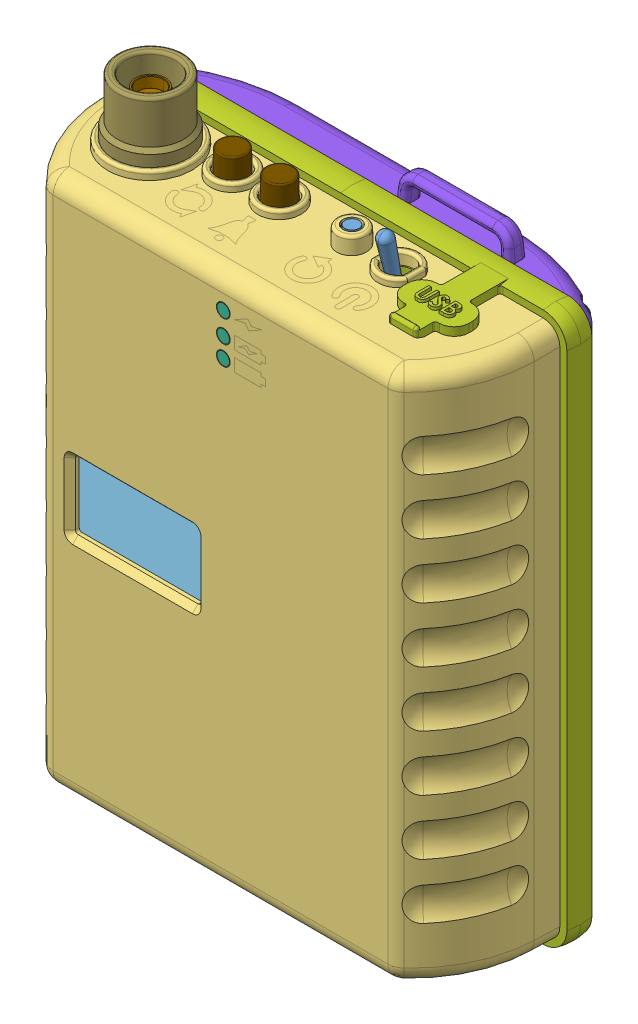
SolidWorks assembly TinyShuffle v.0, configuration Default. Lengths in mm.
Overall size (88.88 109.34 34.5).
53 component instances, 22 part files, 62 mates.
Components (placement in the parent):
- TinyShuffle PCBA v.0a-1: TinyShuffle PCBA v.0a [Default] at (-32.5 0 0) size (65 99.92 17.1)
- SWARM M138-1: SWARM M138 [Default] at (-32.6074 -0.0785 -0.4335) x (1 0 0) z (0 0 1) size (30 50.95 5.16)
- TinyShuffle TOP v.0-2: TinyShuffle TOP v.0 [Default] at origin size (87.38 99.33 23.32)
  - TinyShuffle TOP v.0-1: TinyShuffle TOP v.0 [Default] at origin size (87.38 99.33 23.15)
  - 94459A110_Heat-Set Inserts for Plastic m2X2.5-1: 94459A110_Heat-Set Inserts for Plastic m2X2.5 [94459A110] at (-36.2 89.5 -10.75) x (1 0 0) z (0 1 0) size (3.69 2.8 3.69)
  - 94459A110_Heat-Set Inserts for Plastic m2X2.5-2: 94459A110_Heat-Set Inserts for Plastic m2X2.5 [94459A110] at (36.2 89.5 -10.75) x (1 0 0) z (0 1 0) size (3.69 2.8 3.69)
  - 94459A110_Heat-Set Inserts for Plastic m2X2.5-3: 94459A110_Heat-Set Inserts for Plastic m2X2.5 [94459A110] at (36.2 44.25 -10.75) x (1 0 0) z (0 1 0) size (3.69 2.8 3.69)
  - 94459A110_Heat-Set Inserts for Plastic m2X2.5-4: 94459A110_Heat-Set Inserts for Plastic m2X2.5 [94459A110] at (36.2 -1 -10.75) x (1 0 0) z (0 1 0) size (3.69 2.8 3.69)
  - 94459A110_Heat-Set Inserts for Plastic m2X2.5-5: 94459A110_Heat-Set Inserts for Plastic m2X2.5 [94459A110] at (-36.2 -1 -10.75) x (1 0 0) z (0 1 0) size (3.69 2.8 3.69)
  - 94459A110_Heat-Set Inserts for Plastic m2X2.5-6: 94459A110_Heat-Set Inserts for Plastic m2X2.5 [94459A110] at (-36.2 44.25 -10.75) x (1 0 0) z (0 1 0) size (3.69 2.8 3.69)
  - TinyShuffle Display filter v.0-1: TinyShuffle Display filter v.0 [Default] at origin size (26.56 16.22 2.09)
  - BIVAR PLPC2-8MM-2: BIVAR PLPC2-8MM [Default] at (0.5 82.5 1.9) size (2.28 2.26 8.02)
  - BIVAR PLPC2-8MM-3: BIVAR PLPC2-8MM [Default] at (0.5 79 1.9) size (2.28 2.26 8.02)
  - BIVAR PLPC2-8MM-4: BIVAR PLPC2-8MM [Default] at (0.5 86.5 1.9) size (2.28 2.26 8.02)
  - 94459A110_Heat-Set Inserts for Plastic m2X2.5-7: 94459A110_Heat-Set Inserts for Plastic m2X2.5 [94459A110] at (29.5 75 2.5) x (1 0 0) z (0 1 0) size (3.69 2.8 3.69)
  - 94459A110_Heat-Set Inserts for Plastic m2X2.5-8: 94459A110_Heat-Set Inserts for Plastic m2X2.5 [94459A110] at (1 75 2.5) x (1 0 0) z (0 1 0) size (3.69 2.8 3.69)
  - 94459A110_Heat-Set Inserts for Plastic m2X2.5-9: 94459A110_Heat-Set Inserts for Plastic m2X2.5 [94459A110] at (-29.5 75 2.5) x (1 0 0) z (0 1 0) size (3.69 2.8 3.69)
  - 94459A110_Heat-Set Inserts for Plastic m2X2.5-10: 94459A110_Heat-Set Inserts for Plastic m2X2.5 [94459A110] at (-29.5 3 2.5) x (1 0 0) z (0 1 0) size (3.69 2.8 3.69)
  - 94459A110_Heat-Set Inserts for Plastic m2X2.5-11: 94459A110_Heat-Set Inserts for Plastic m2X2.5 [94459A110] at (29.5 3 2.5) x (1 0 0) z (0 1 0) size (3.69 2.8 3.69)
- TinyShuffle SHIM v.0-1: TinyShuffle SHIM v.0 [Default] at origin size (82 100.03 19.68)
- TinyShuffle BOT v.0-1: TinyShuffle BOT v.0 [Default] at origin size (79 101.5 24.59)
- SMA_CONNECTOR-1: SMA_CONNECTOR [Default] at (-26 101.6 -3.5) x (0 0 1) z (0 1 0) size (8.14 9.4 22.5)
- TYPE-C JACK-1: TYPE-C JACK [Default] at (26.205 88.375 -3.0876) x (0 0 1) z (0 1 0) size (6 10 35.27) (hidden)
- Swarm-1_4-wave-antenna-model-1: Swarm-1_4-wave-antenna-model [Default] at (-26 96.7375 -3.5) x (-1 0 0) z (0 1 0) size (11.04 11.04 215.14) (hidden)
- SMA_WASHER-1: SMA_WASHER [Default] at (-26 93 -3.5) x (1 0 0) z (0 -1 0) size (9 9 0.5)
- NT-SMA-N-1: NT-SMA-N [Default] at (-26 93.85 -3.5) x (0.997814 0 -0.066084) z (0 -1 0) size (9.24 8 1.7)
- TinyShuffle SMA SEAL v.0-1: TinyShuffle SMA SEAL v.0 [Default] at origin size (13.22 11.59 13.22)
- 92095A452_Button Head Hex Drive Screw M2x5-1: 92095A452_Button Head Hex Drive Screw M2x5 [92095A452] at (-27.3953 53.0669 5.935) size (3.5 3.5 6.52)
- 92095A452_Button Head Hex Drive Screw M2x5-2: 92095A452_Button Head Hex Drive Screw M2x5 [92095A452] at (-4.2953 53.0669 5.935) x (0.482092 -0.876121 0) z (0 0 1) size (3.5 3.5 6.52)
- 92095A452_Button Head Hex Drive Screw M2x5-3: 92095A452_Button Head Hex Drive Screw M2x5 [92095A452] at (-27.3953 29.5069 5.935) x (0.482092 -0.876121 0) z (0 0 1) size (3.5 3.5 6.52)
- 92095A452_Button Head Hex Drive Screw M2x5-4: 92095A452_Button Head Hex Drive Screw M2x5 [92095A452] at (-4.2953 29.5069 5.935) x (0.482092 -0.876121 0) z (0 0 1) size (3.5 3.5 6.52)
- 93475A195_18-8 Stainless Steel Washer M2X5-1: 93475A195_18-8 Stainless Steel Washer M2X5 [93475A195] at (29.5 75 -1.99) size (5 5 0.4)
- 93475A195_18-8 Stainless Steel Washer M2X5-2: 93475A195_18-8 Stainless Steel Washer M2X5 [93475A195] at (1 75 -1.99) size (5 5 0.4)
- 93475A195_18-8 Stainless Steel Washer M2X5-3: 93475A195_18-8 Stainless Steel Washer M2X5 [93475A195] at (-29.5 75 -1.99) size (5 5 0.4)
- 93475A195_18-8 Stainless Steel Washer M2X5-4: 93475A195_18-8 Stainless Steel Washer M2X5 [93475A195] at (-29.5 3 -1.99) size (5 5 0.4)
- 93475A195_18-8 Stainless Steel Washer M2X5-5: 93475A195_18-8 Stainless Steel Washer M2X5 [93475A195] at (29.5 3 -1.99) size (5 5 0.4)
- 92095A452_Button Head Hex Drive Screw M2x5-5: 92095A452_Button Head Hex Drive Screw M2x5 [92095A452] at (29.5 75 -3.29) x (1 0 0) z (0 0 -1) size (3.5 3.5 6.52)
- 92095A452_Button Head Hex Drive Screw M2x5-6: 92095A452_Button Head Hex Drive Screw M2x5 [92095A452] at (1 75 -3.29) x (1 0 0) z (0 0 -1) size (3.5 3.5 6.52)
- 92095A452_Button Head Hex Drive Screw M2x5-7: 92095A452_Button Head Hex Drive Screw M2x5 [92095A452] at (-29.5 75 -3.29) x (1 0 0) z (0 0 -1) size (3.5 3.5 6.52)
- 92095A452_Button Head Hex Drive Screw M2x5-8: 92095A452_Button Head Hex Drive Screw M2x5 [92095A452] at (-29.5 3 -3.29) x (1 0 0) z (0 0 -1) size (3.5 3.5 6.52)
- 92095A452_Button Head Hex Drive Screw M2x5-9: 92095A452_Button Head Hex Drive Screw M2x5 [92095A452] at (29.5 3 -3.29) x (1 0 0) z (0 0 -1) size (3.5 3.5 6.52)
- 92095A454_Button Head Hex Drive Screw M2X8-1: 92095A454_Button Head Hex Drive Screw M2X8 [92095A454] at (36.2 -1 -19.55) x (1 0 0) z (0 0 -1) size (3.5 3.5 9.53)
- 92095A454_Button Head Hex Drive Screw M2X8-2: 92095A454_Button Head Hex Drive Screw M2X8 [92095A454] at (36.2 44.25 -19.55) x (1 0 0) z (0 0 -1) size (3.5 3.5 9.53)
- 92095A454_Button Head Hex Drive Screw M2X8-3: 92095A454_Button Head Hex Drive Screw M2X8 [92095A454] at (36.2 89.5 -19.55) x (1 0 0) z (0 0 -1) size (3.5 3.5 9.53)
- 92095A454_Button Head Hex Drive Screw M2X8-4: 92095A454_Button Head Hex Drive Screw M2X8 [92095A454] at (-36.2 89.5 -19.55) x (1 0 0) z (0 0 -1) size (3.5 3.5 9.53)
- 92095A454_Button Head Hex Drive Screw M2X8-5: 92095A454_Button Head Hex Drive Screw M2X8 [92095A454] at (-36.2 44.25 -19.55) x (1 0 0) z (0 0 -1) size (3.5 3.5 9.53)
- 92095A454_Button Head Hex Drive Screw M2X8-6: 92095A454_Button Head Hex Drive Screw M2X8 [92095A454] at (-36.2 -1 -19.55) x (1 0 0) z (0 0 -1) size (3.5 3.5 9.53)
- 4035N11-1: 4035N11 [Default] at (-5 82.241 -22.209) x (-1 0 0) z (0 0 -1) size (12.7 12.7 0.38)
- W3908B0100-1: W3908B0100 [Default] at (15.25 63.7521 7.58) x (-1 0 0) z (0 0 -1) size (20 26.8 1.45)
- 800AC1BLKCAP-1: 800AC1BLKCAP [Default] at (-14 92.73 -6.27) x (1 0 0) z (0 0 1) size (5 5.03 5)
- 800AC1BLKCAP-2: 800AC1BLKCAP [Default] at (-5.5 92.73 -6.27) x (1 0 0) z (0 0 1) size (5 5.03 5)
- 353 Adafruit battery-1: 353 Adafruit battery [Default] at (-32.5 0.5 1) x (1 0 0) z (0 0 1) size (54 70 18)
- 3M 4026 FOAM .0625IN THICK-1: 3M 4026 FOAM .0625IN THICK [Default] at (-32.5 0.5 -20.59) x (-1 0 0) z (0 0 -1) size (35 65 1.59)
Mates (geometry in assembly coordinates):
- Coincident1: coincident: plane of assembly through (0 0 0) normal (0 0 1); plane of TinyShuffle PCBA v.0a-1 through (-32.5 0 0) normal (0 0 1); plane of assembly
- Symmetric1: symmetric: plane of assembly; plane of assembly; plane of TinyShuffle PCBA v.0a-1 through (-32.5 83.5 -1.59) normal (-1 0 0); plane of TinyShuffle PCBA v.0a-1 through (32.5 1 -1.59) normal (1 0 0); plane of assembly
- Coincident2: coincident: plane of assembly through (0 0 0) normal (0 1 0); plane of TinyShuffle PCBA v.0a-1 through (-32.5 0 0) normal (0 1 0); plane of assembly
- Parallel1: parallel aligned: plane of SMA_CONNECTOR-1 through (-27.5098 90.5 -0.7358) normal (0 0 1)
- Parallel2: parallel aligned: plane of SMA_CONNECTOR-1 through (-26 101.6 -3.5) normal (0 1 0)
- Distance1: distance = 3.5 mm aligned: plane of SMA_CONNECTOR-1 through (-26 101.6 -3.5) normal (0 0 1)
- Distance2: distance = 26 mm: plane of assembly through (0 0 0) normal (1 0 0); plane of assembly; plane of SMA_CONNECTOR-1 through (-26 101.6 -3.5) normal (1 0 0)
- Distance3: distance = 3.35 mm: plane of TinyShuffle PCBA v.0a-1 through (26.205 91.675 -3.0876) normal (0 1 0); plane of TYPE-C JACK-1 through (24.205 95.025 -3.0876) normal (0 -1 0)
- Width1: width: plane of TYPE-C JACK-1 through (24.205 110.025 -6.0876) normal (0 0 -1); plane of TYPE-C JACK-1 through (24.205 110.025 -0.0876) normal (0 0 1); plane of TinyShuffle PCBA v.0a-1 through (26.205 89.375 -4.3676) normal (0 0 1); plane of TinyShuffle PCBA v.0a-1 through (26.205 89.375 -1.8076) normal (0 0 -1)
- Distance4: distance = 26.205 mm: plane of assembly; plane of TYPE-C JACK-1 through (26.205 88.375 -3.0876) normal (1 0 0); point of assembly
- Concentric1: concentric: circle of SMA_CONNECTOR-1; circle of Swarm-1_4-wave-antenna-model-1
- Coincident3: coincident: plane of SMA_CONNECTOR-1 through (-26 99.5696 -3.5) normal (0 1 0); point of Swarm-1_4-wave-antenna-model-1
- Parallel3: parallel: plane of assembly through (0 0 0) normal (1 0 0); plane of Swarm-1_4-wave-antenna-model-1 through (-26 96.7375 -3.5) normal (-1 0 0); plane of assembly
- Concentric3: concentric anti-aligned: cone of TinyShuffle PCBA v.0a-1 through (-27.4 53.07 3.25) axis (0 0 -1); cylinder of pan head cross recess screw_iso-1 through (-27.4 53.07 31.635) axis (0 0 1) radius 2
- Coincident5: coincident anti-aligned: plane of TinyShuffle PCBA v.0a-1 through (-4.2953 53.0669 4.635) normal (0 0 1); plane of pan head cross recess screw_iso-1 through (-27.4 54.07 4.635) normal (0 0 -1)
- Concentric4: concentric: circle of TinyShuffle PCBA v.0-1; circle of 92095A452_Button Head Hex Drive Screw M2x5-1
- Coincident6: coincident: plane of TinyShuffle PCBA v.0a-1 through (-27.3953 53.0669 4.635) normal (0 0 1); circle of 92095A452_Button Head Hex Drive Screw M2x5-1
- Concentric5: concentric: circle of TinyShuffle PCBA v.0-1; circle of 92095A452_Button Head Hex Drive Screw M2x5-2
- Coincident7: coincident: plane of TinyShuffle PCBA v.0a-1 through (-4.2953 53.0669 4.635) normal (0 0 1); circle of 92095A452_Button Head Hex Drive Screw M2x5-2
- Coincident8: coincident: plane of TinyShuffle PCBA v.0a-1 through (-27.3953 29.5069 4.635) normal (0 0 1); circle of 92095A452_Button Head Hex Drive Screw M2x5-3
- Concentric6: concentric: circle of TinyShuffle PCBA v.0-1; circle of 92095A452_Button Head Hex Drive Screw M2x5-3
- Coincident9: coincident: plane of TinyShuffle PCBA v.0a-1 through (-4.2953 29.5069 4.635) normal (0 0 1); circle of 92095A452_Button Head Hex Drive Screw M2x5-4
- Concentric7: concentric: circle of TinyShuffle PCBA v.0-1; circle of 92095A452_Button Head Hex Drive Screw M2x5-4
- Concentric8: concentric aligned: circle of SMA_CONNECTOR-1; circle of SMA_WASHER-1
- Concentric9: concentric: circle of SMA_WASHER-1; circle of NT-SMA-N-1
- Coincident10: coincident: plane of SMA_WASHER-1 through (-26 93 -3.5) normal (0 1 0); plane of NT-SMA-N-1 through (-26 93 -3.5) normal (0 -1 0)
- ProfileCenter2: profile center: circle of 93475A195_18-8 Stainless Steel Washer M2X5-1; circle of TinyShuffle PCBA v.0-1
- ProfileCenter3: profile center: circle of 93475A195_18-8 Stainless Steel Washer M2X5-2; circle of TinyShuffle PCBA v.0-1
- ProfileCenter4: profile center: circle of 93475A195_18-8 Stainless Steel Washer M2X5-3; circle of TinyShuffle PCBA v.0-1
- ProfileCenter5: profile center: circle of 93475A195_18-8 Stainless Steel Washer M2X5-4; circle of TinyShuffle PCBA v.0-1
- ProfileCenter6: profile center: circle of 93475A195_18-8 Stainless Steel Washer M2X5-5; circle of TinyShuffle PCBA v.0-1
- ProfileCenter7: profile center: circle of 92095A452_Button Head Hex Drive Screw M2x5-5; circle of 93475A195_18-8 Stainless Steel Washer M2X5-1
- ProfileCenter8: profile center: circle of 92095A452_Button Head Hex Drive Screw M2x5-6; circle of 93475A195_18-8 Stainless Steel Washer M2X5-2
- ProfileCenter9: profile center: circle of 92095A452_Button Head Hex Drive Screw M2x5-7; circle of 93475A195_18-8 Stainless Steel Washer M2X5-3
- ProfileCenter10: profile center: circle of 92095A452_Button Head Hex Drive Screw M2x5-8; circle of 93475A195_18-8 Stainless Steel Washer M2X5-4
- ProfileCenter11: profile center: circle of 92095A452_Button Head Hex Drive Screw M2x5-9; circle of 93475A195_18-8 Stainless Steel Washer M2X5-5
- ProfileCenter12: profile center: circle of TinyShuffle BOT v.0-1; circle of 92095A454_Button Head Hex Drive Screw M2X8-1
- ProfileCenter13: profile center: circle of 92095A454_Button Head Hex Drive Screw M2X8-2; circle of TinyShuffle BOT v.0-1
- ProfileCenter14: profile center: circle of TinyShuffle BOT v.0-1; circle of 92095A454_Button Head Hex Drive Screw M2X8-3
- ProfileCenter15: profile center: circle of 92095A454_Button Head Hex Drive Screw M2X8-4; circle of TinyShuffle BOT v.0-1
- ProfileCenter16: profile center: circle of 92095A454_Button Head Hex Drive Screw M2X8-5; circle of TinyShuffle BOT v.0-1
- ProfileCenter17: profile center: circle of 92095A454_Button Head Hex Drive Screw M2X8-6; circle of TinyShuffle BOT v.0-1
- ProfileCenter18: profile center: circle of 4035N11-1; circle of TinyShuffle BOT v.0-1
- Coincident11: coincident: plane of TinyShuffle TOP v.0-2/TinyShuffle TOP v.0-1 through (31.3034 92.5 7.9) normal (0 0 -1); plane of W3908B0100-1 through (15.25 63.7521 7.9) normal (0 0 1)
- Parallel4: parallel aligned: line of TinyShuffle TOP v.0-2/TinyShuffle TOP v.0-1 through (30.1533 5.7617 7.9022) axis (0 1 0); line of W3908B0100-1 through (25.25 87.1736 7.9022) axis (-1 0 0)
- Parallel5: parallel: line of TinyShuffle TOP v.0-2/TinyShuffle TOP v.0-1 through (-33.5 90.5 -13.25) axis (1 0 0); line of W3908B0100-1 through (5.25 77.1521 7.58) axis (1 0 0)
- Distance5: distance = 12 mm: line of TinyShuffle TOP v.0-2/TinyShuffle TOP v.0-1 through (30.1556 89.1478 7.9) axis (-1 0 0); line of W3908B0100-1 through (5.25 77.1521 7.58) axis (1 0 0)
- Distance6: distance = 14.25 mm: plane of W3908B0100-1 through (15.25 63.7521 7.58) normal (-1 0 0); unknown of ?
- Coincident12: coincident: plane of TinyShuffle PCBA v.0a-1 through (-12.603 95.33 -7.667) normal (0 1 0); plane of 800AC1BLKCAP-1 through (-14 95.33 -5.62) normal (0 -1 0)
- Concentric10: concentric: circle of TinyShuffle PCBA v.0a-1; cone of 800AC1BLKCAP-1 through (-14 96.76 -6.27) axis (0 1 0)
- Coincident13: coincident: plane of TinyShuffle PCBA v.0a-1 through (-4.103 95.33 -7.667) normal (0 1 0); plane of 800AC1BLKCAP-2 through (-5.5 95.33 -5.62) normal (0 -1 0)
- Concentric11: concentric: circle of TinyShuffle PCBA v.0a-1; cone of 800AC1BLKCAP-2 through (-5.5 96.76 -6.27) axis (0 1 0)
- Concentric12: concentric: circle of TinyShuffle PCBA v.0a-1; circle of SWARM M138-1
- Width2: width: plane of TinyShuffle PCBA v.0a-1 through (0.2088 62.6755 1.1) normal (0 0 1); plane of TinyShuffle PCBA v.0a-1 through (27.6088 66.7755 2.5) normal (0 0 -1); plane of SWARM M138-1 through (27.5588 15.7365 1.3345) normal (0 0 -1); plane of SWARM M138-1 through (27.5588 15.7365 2.2655) normal (0 0 1)
- Concentric13: concentric: circle of TinyShuffle PCBA v.0a-1; circle of SWARM M138-1
- Distance7: distance = 1 mm: plane of 353 Adafruit battery-1 through (0 35.5 -2.59) normal (0 0 1); plane of TinyShuffle PCBA v.0a-1 through (-32.5 1 -1.59) normal (0 0 -1)
- Symmetric2: symmetric: cylinder of assembly; cylinder of assembly; cylinder of 353 Adafruit battery-1 through (-18 18 -11.59) axis (0 1 0) radius 9; cylinder of 353 Adafruit battery-1 through (18 53 -11.59) axis (0 -1 0) radius 9; plane of assembly
- Distance8: distance = 0.5 mm: plane of 353 Adafruit battery-1 through (27 0.5 -2.59) normal (0 -1 0); plane of TinyShuffle PCBA v.0a-1 through (-31.5 0 -1.59) normal (0 -1 0)
- InPlace1: in place: plane of 353 Adafruit battery-1 through (0 35.5 -20.59) normal (0 0 -1); plane of ? through (0 0 -20.59) normal (0 0 -1); moOrthogonalPlaneRef_w of 353 Adafruit battery-1 through (0 35.5 -20.59) normal (0 0 -1); plane of ? through (0 0 -20.59) normal (0 1 0); plane of 353 Adafruit battery-1 through (0 35.5 -20.59) normal (0 0 -1); plane of ? through (0 0 -20.59) normal (-1 0 0); plane of 353 Adafruit battery-1 through (0 35.5 -20.59) normal (0 0 -1); unknown of 3M 4026 FOAM .0625IN THICK-1
- Coincident14: coincident: plane of ?; plane of ?
- Coincident15: coincident: moOrthogonalPlaneRef_w of 353 Adafruit battery-1 through (-32.5 0.5 -20.59) normal (0 1 0); plane of Part1^TinyShuffle v.0-1 through (-32.5 0.5 -20.59) normal (0 1 0)
- Coincident16: coincident: moOrthogonalPlaneRef_w of 353 Adafruit battery-1 through (-32.5 0.5 -20.59) normal (1 0 0); plane of Part1^TinyShuffle v.0-1 through (-32.5 0.5 -20.59) normal (-1 0 0)
